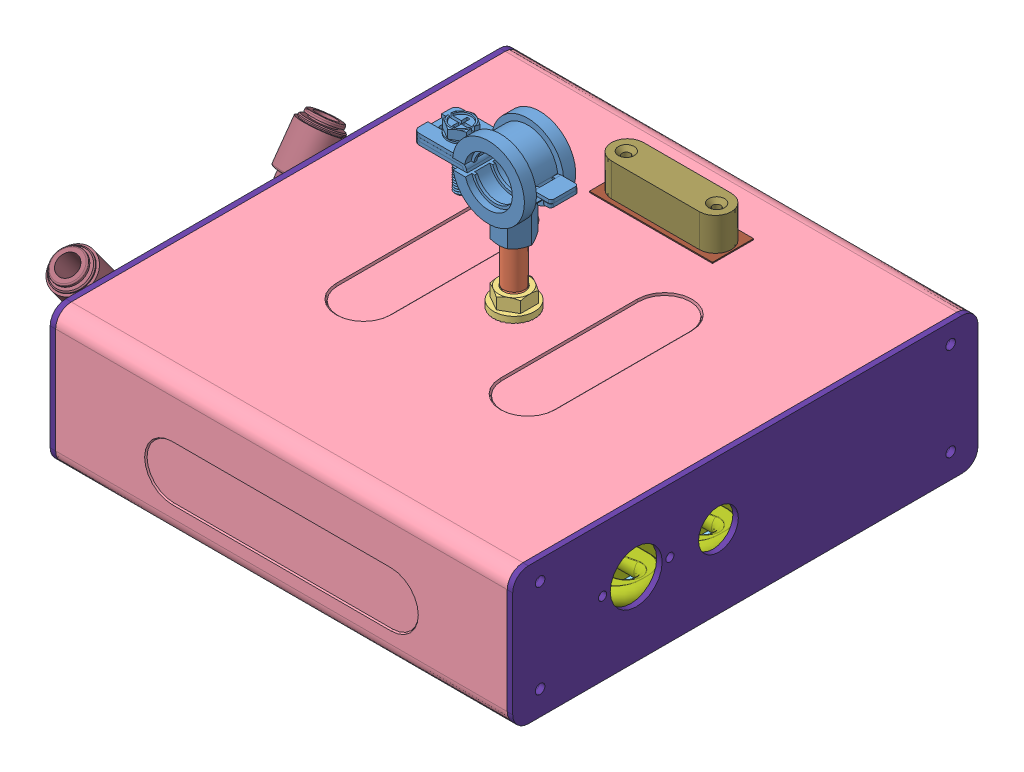
SolidWorks assembly LFR.101, configuration Default. Lengths in mm.
Overall size (264.18 207.36 215.9).
37 component instances, 17 part files, 61 mates.
Components (placement in the parent):
- 2615T130_VIBRATION-DAMPING CLAMPING HANGER-1: 2615T130_VIBRATION-DAMPING CLAMPING HANGER [2615T13] x (-1 0 0) z (0 0 1) size (60.33 44.72 23.81)
- 92386A632_SS THRD-LOCKING ADJUSTING   POSITIONING STUD-1: 92386A632_SS THRD-LOCKING ADJUSTING   POSITIONING STUD [92386A632] at (0 -65.8495 0) x (1 0 0) z (0 -1 0) size (10.08 10.01 51.87)
- 93776A461_TYPE 18-8 SS SERRATED-FLANGE LOCKNUT-1: 93776A461_TYPE 18-8 SS SERRATED-FLANGE LOCKNUT [93776A461] at (0 -47.3075 0) x (1 0 0) z (0 1 0) size (19.05 19.05 9.51)
- LFR.001-1: LFR.001 [BENT] at (0 -56.0388 0) size (209.55 64.1 215.9)
- LightPanel-1: LightPanel [Default] at (5.3651 -116.5988 -8.8508) x (0 0 -1) z (-1 0 0) size (195.78 12.57 210.82)
  - LightPCB-1: LightPCB [Default] at (-97.8524 -1.8098 101.8851) size (195.78 1.57 210.82)
  - KNAC36xxADS_Optic-1: KNAC36xxADS_Optic [Default] at (-8.8508 2.765 90.5129) x (0 0 1) z (0 1 0) size (193.04 178 11)
- aavid_heatsink-1: aavid_heatsink [Default] at (0.2 -114.7889 0) x (-1 0 0) z (0 0 -1) size (237.85 17.03 177.8)
- 92949A133_18-8 SS BUTTON-HEAD SOCKET CAP SCREW-1: 92949A133_18-8 SS BUTTON-HEAD SOCKET CAP SCREW [92949A133] at (100.965 -121.2151 93.4466) x (-0.331806 0 0.943348) z (0 -1 0) size (6.05 6.05 11.55)
- 94241A230_TYPE 316 STAINLESS STEEL SPLIT LOCK WASHER-1: 94241A230_TYPE 316 STAINLESS STEEL SPLIT LOCK WASHER [94241A230] at (100.965 -114.0269 93.4466) x (0.331806 0 -0.943348) z (0 -1 0) size (5.13 5.14 1.64)
- 90730A006_TYPE 18-8 STAINLESS STEEL NARROW HEX NUT-1: 90730A006_TYPE 18-8 STAINLESS STEEL NARROW HEX NUT [90730A006] at (100.965 -111.9978 93.4466) x (0.975805 0 0.218641) z (-0.218641 0 0.975805) size (6.35 2.87 7.33)
- 92949A133_18-8 SS BUTTON-HEAD SOCKET CAP SCREW-4: 92949A133_18-8 SS BUTTON-HEAD SOCKET CAP SCREW [92949A133] at (-100.965 -121.2151 93.4466) x (-0.331806 0 0.943348) z (0 -1 0) size (6.05 6.05 11.55)
- 92949A133_18-8 SS BUTTON-HEAD SOCKET CAP SCREW-5: 92949A133_18-8 SS BUTTON-HEAD SOCKET CAP SCREW [92949A133] at (100.965 -121.2151 -94.0054) x (-0.331806 0 0.943348) z (0 -1 0) size (6.05 6.05 11.55)
- 92949A133_18-8 SS BUTTON-HEAD SOCKET CAP SCREW-8: 92949A133_18-8 SS BUTTON-HEAD SOCKET CAP SCREW [92949A133] at (-100.965 -121.2151 -94.0054) x (-0.331806 0 0.943348) z (0 -1 0) size (6.05 6.05 11.55)
- 90730A006_TYPE 18-8 STAINLESS STEEL NARROW HEX NUT-4: 90730A006_TYPE 18-8 STAINLESS STEEL NARROW HEX NUT [90730A006] at (-100.965 -111.9978 93.4466) x (0.975805 0 0.218641) z (-0.218641 0 0.975805) size (6.35 2.87 7.33)
- 90730A006_TYPE 18-8 STAINLESS STEEL NARROW HEX NUT-5: 90730A006_TYPE 18-8 STAINLESS STEEL NARROW HEX NUT [90730A006] at (100.965 -111.9978 -94.0054) x (0.975805 0 0.218641) z (-0.218641 0 0.975805) size (6.35 2.87 7.33)
- 90730A006_TYPE 18-8 STAINLESS STEEL NARROW HEX NUT-8: 90730A006_TYPE 18-8 STAINLESS STEEL NARROW HEX NUT [90730A006] at (-100.965 -111.9978 -94.0054) x (0.975805 0 0.218641) z (-0.218641 0 0.975805) size (6.35 2.87 7.33)
- 94241A230_TYPE 316 STAINLESS STEEL SPLIT LOCK WASHER-4: 94241A230_TYPE 316 STAINLESS STEEL SPLIT LOCK WASHER [94241A230] at (-100.965 -114.0269 93.4466) x (0.331806 0 -0.943348) z (0 -1 0) size (5.13 5.14 1.64)
- 94241A230_TYPE 316 STAINLESS STEEL SPLIT LOCK WASHER-5: 94241A230_TYPE 316 STAINLESS STEEL SPLIT LOCK WASHER [94241A230] at (100.965 -114.0269 -94.0054) x (0.331806 0 -0.943348) z (0 -1 0) size (5.13 5.14 1.64)
- 94241A230_TYPE 316 STAINLESS STEEL SPLIT LOCK WASHER-8: 94241A230_TYPE 316 STAINLESS STEEL SPLIT LOCK WASHER [94241A230] at (-100.965 -114.0269 -94.0054) x (0.331806 0 -0.943348) z (0 -1 0) size (5.13 5.14 1.64)
- 76665A68_VHB_TAPE-1: 76665A68_VHB_TAPE [Default] at (0 -56.0388 -73.025) x (0 0 1) z (-1 0 0) size (19.05 0.51 57.15)
- 3338A22_HORIZONTAL_SURFACE_MOUNT_LEVEL-1: 3338A22_HORIZONTAL_SURFACE_MOUNT_LEVEL [Default] at (0.0625 -55.5307 -72.9641) size (55.63 15.24 14.83)
- 9406T170_PUSH-TO-CONNECT TUBE FITTING FOR SS TUBING-1: 9406T170_PUSH-TO-CONNECT TUBE FITTING FOR SS TUBING [9406T17] at (-147.214 -103.439 -45.2) x (0 -0.582087 -0.813127) z (1 0 0) size (19.3 35.05 39.88)
- 9406T170_PUSH-TO-CONNECT TUBE FITTING FOR SS TUBING-2: 9406T170_PUSH-TO-CONNECT TUBE FITTING FOR SS TUBING [9406T17] at (-147.214 -103.439 45) x (0 0.587828 -0.808986) z (1 0 0) size (19.3 35.05 39.88)
- 94639A303_NYLON UNTHREADED SPACERS-1: 94639A303_NYLON UNTHREADED SPACERS [94639A303] at (-40.44 -94.4389 -55.499) x (0.961212 0 0.275811) z (0 1 0) size (6.35 6.35 12.7)
- 94639A303_NYLON UNTHREADED SPACERS-2: 94639A303_NYLON UNTHREADED SPACERS [94639A303] at (40.84 -94.4389 -55.499) x (0.961212 0 0.275811) z (0 1 0) size (6.35 6.35 12.7)
- 94639A303_NYLON UNTHREADED SPACERS-3: 94639A303_NYLON UNTHREADED SPACERS [94639A303] at (40.84 -94.4389 55.499) x (0.961212 0 0.275811) z (0 1 0) size (6.35 6.35 12.7)
- 94639A303_NYLON UNTHREADED SPACERS-4: 94639A303_NYLON UNTHREADED SPACERS [94639A303] at (-40.44 -94.4389 55.499) x (0.961212 0 0.275811) z (0 1 0) size (6.35 6.35 12.7)
- 92949A151_18-8 SS BUTTON-HEAD SOCKET CAP SCREW-1: 92949A151_18-8 SS BUTTON-HEAD SOCKET CAP SCREW [92949A151] at (-40.44 -84.4567 -55.499) x (0.994916 0 -0.100706) z (0 1 0) size (6.65 6.65 21.35)
- 92949A151_18-8 SS BUTTON-HEAD SOCKET CAP SCREW-2: 92949A151_18-8 SS BUTTON-HEAD SOCKET CAP SCREW [92949A151] at (-40.44 -84.4567 55.499) x (0.991359 0 -0.131179) z (0 1 0) size (6.65 6.65 21.35)
- 92949A151_18-8 SS BUTTON-HEAD SOCKET CAP SCREW-3: 92949A151_18-8 SS BUTTON-HEAD SOCKET CAP SCREW [92949A151] at (40.84 -84.4567 55.499) x (0.991359 0 -0.131179) z (0 1 0) size (6.65 6.65 21.35)
- 92949A151_18-8 SS BUTTON-HEAD SOCKET CAP SCREW-4: 92949A151_18-8 SS BUTTON-HEAD SOCKET CAP SCREW [92949A151] at (40.84 -84.4567 -55.499) x (0.991359 0 -0.131179) z (0 1 0) size (6.65 6.65 21.35)
- light_controller v16-1: light_controller v16 [Default] at (-45.52 -88.0889 -60.579) x (0 0 1) z (0 1 0) size (121.16 91.44 17.03)
- LFR.008-1: LFR.008 [Front-1] at (-102.235 -158.9087 0) x (0 0 1) z (-1 0 0) size (215.9 131.44 2.54)
- LFR.008-2: LFR.008 [Front-2] at (-104.775 -87.7887 0) x (0 0 1) z (-1 0 0) size (215.9 131.44 2.54)
- LFR.008-3: LFR.008 [Back1] at (104.775 -158.9087 0) x (0 0 1) z (-1 0 0) size (215.9 131.44 2.54)
- LFR.008-4: LFR.008 [Back2] at (107.315 -87.7887 0) x (0 0 1) z (-1 0 0) size (215.9 131.44 2.54)
Mates (geometry in assembly coordinates):
- Coincident1: coincident: plane of 2615T130_VIBRATION-DAMPING CLAMPING HANGER-1 through (0 0 0) normal (0 0 1); plane of assembly through (0 0 0) normal (0 0 1)
- Coincident2: coincident: plane of 2615T130_VIBRATION-DAMPING CLAMPING HANGER-1 through (0 0 0) normal (0 -1 0); plane of assembly through (0 0 0) normal (0 1 0)
- Coincident3: coincident: plane of 2615T130_VIBRATION-DAMPING CLAMPING HANGER-1 through (0 0 0) normal (-1 0 0); plane of assembly through (0 0 0) normal (1 0 0)
- Concentric1: concentric: cylinder of 2615T130_VIBRATION-DAMPING CLAMPING HANGER-1 through (0 16.7015 0) axis (0 -1 0) radius 5.3975; cylinder of 92386A632_SS THRD-LOCKING ADJUSTING   POSITIONING STUD-1 through (0 -15.0495 0) axis (0 1 0) radius 4.7625
- Coincident4: coincident: plane of 2615T130_VIBRATION-DAMPING CLAMPING HANGER-1 through (-8.1389 -27.7495 0) normal (0 -1 0); plane of 92386A632_SS THRD-LOCKING ADJUSTING   POSITIONING STUD-1 through (0 -27.7495 0) normal (0 1 0)
- Concentric2: concentric: cylinder of LFR.001-1 through (0 -59.2138 0) axis (0 -1 0) radius 7.112; cylinder of 92386A632_SS THRD-LOCKING ADJUSTING   POSITIONING STUD-1 through (0 -15.0495 0) axis (0 1 0) radius 4.7625
- Concentric3: concentric: cylinder of 93776A461_TYPE 18-8 SS SERRATED-FLANGE LOCKNUT-1 through (0 -53.0669 0) axis (0 -1 0) radius 9.525; cylinder of 92386A632_SS THRD-LOCKING ADJUSTING   POSITIONING STUD-1 through (0 -15.0495 0) axis (0 1 0) radius 4.7625
- Coincident5: coincident: plane of LFR.001-1 through (-104.775 -56.0388 107.95) normal (0 1 0); point of 93776A461_TYPE 18-8 SS SERRATED-FLANGE LOCKNUT-1
- Parallel1: parallel: plane of 2615T130_VIBRATION-DAMPING CLAMPING HANGER-1 through (-36.83 -3.1877 33.5953) normal (-1 0 0); plane of LFR.001-1 through (-104.775 -59.2138 107.95) normal (-1 0 0)
- Distance1: distance = 0.508 mm: plane of 93776A461_TYPE 18-8 SS SERRATED-FLANGE LOCKNUT-1 through (-7.1437 -47.3075 -12.3733) normal (0 1 0); plane of 92386A632_SS THRD-LOCKING ADJUSTING   POSITIONING STUD-1 through (0 -46.7995 0) normal (0 -1 0)
- Coincident6: coincident: plane of LightPanel-1/LightPCB-1 through (-96.52 -114.7889 89.0016) normal (0 1 0); plane of aavid_heatsink-1 through (0.2 -114.7889 0) normal (0 -1 0)
- Distance2: distance = 29.21 mm: plane of aavid_heatsink-1 through (76.2 -100.7889 88.9) normal (1 0 0); plane of LightPanel-1/LightPCB-1 through (105.41 -116.3637 -97.8916) normal (1 0 0)
- Coincident8: coincident: plane of LFR.001-1 through (0 -116.3637 0) normal (0 1 0); plane of LightPanel-1/LightPCB-1 through (-96.52 -116.3637 89.0016) normal (0 -1 0)
- Width3: width: plane of aavid_heatsink-1 through (76.2 -100.7889 -88.9) normal (0 0 -1); plane of aavid_heatsink-1 through (76.2 -100.7889 88.9) normal (0 0 1); plane of LightPanel-1/LightPCB-1 through (105.41 -116.3637 97.8916) normal (0 0 1); plane of LightPanel-1/LightPCB-1 through (-105.41 -116.3637 -97.8916) normal (0 0 -1)
- Parallel2: parallel: plane of LFR.001-1 through (104.775 -56.0388 107.95) normal (1 0 0); plane of aavid_heatsink-1 through (76.2 -100.7889 88.9) normal (1 0 0)
- Width4: width: plane of LFR.001-1 through (0 -56.0388 107.95) normal (0 0 1); plane of LFR.001-1 through (0 -56.0388 -107.95) normal (0 0 -1); plane of aavid_heatsink-1 through (76.2 -100.7889 -88.9) normal (0 0 -1); plane of aavid_heatsink-1 through (76.2 -100.7889 88.9) normal (0 0 1)
- Width5: width: plane of LightPanel-1/LightPCB-1 through (105.41 -116.3637 -97.8916) normal (1 0 0); plane of LightPanel-1/LightPCB-1 through (-105.41 -116.3637 97.8916) normal (-1 0 0); plane of LFR.001-1 through (104.775 -59.2138 107.95) normal (1 0 0); plane of LFR.001-1 through (-104.775 -119.5387 107.95) normal (-1 0 0)
- Concentric4: concentric: cylinder of LightPanel-1/LightPCB-1 through (100.965 -116.3637 93.4466) axis (0 1 0) radius 1.778; cylinder of 92949A133_18-8 SS BUTTON-HEAD SOCKET CAP SCREW-1 through (100.965 -121.2151 93.4466) axis (0 -1 0) radius 3.0226
- Coincident11: coincident: plane of LightPanel-1/LightPCB-1 through (-96.52 -114.7889 89.0016) normal (0 1 0); point of 94241A230_TYPE 316 STAINLESS STEEL SPLIT LOCK WASHER-1
- Parallel3: parallel: plane of LightPanel-1/LightPCB-1 through (-96.52 -114.7889 89.0016) normal (0 1 0); plane of 94241A230_TYPE 316 STAINLESS STEEL SPLIT LOCK WASHER-1 through (100.965 -114.0269 93.4466) normal (0 -1 0)
- Coincident13: coincident: plane of 92949A133_18-8 SS BUTTON-HEAD SOCKET CAP SCREW-1 through (100.965 -121.2151 93.4466) normal (-0.331806 0 0.943348); plane of 94241A230_TYPE 316 STAINLESS STEEL SPLIT LOCK WASHER-1 through (100.965 -114.0269 93.4466) normal (0.331806 0 -0.943348)
- Coincident14: coincident: plane of 92949A133_18-8 SS BUTTON-HEAD SOCKET CAP SCREW-1 through (100.965 -121.2151 93.4466) normal (-0.943348 0 -0.331806); plane of 94241A230_TYPE 316 STAINLESS STEEL SPLIT LOCK WASHER-1 through (100.965 -114.0269 93.4466) normal (0.943348 0 0.331806)
- Coincident15: coincident: plane of LFR.001-1 through (0 -119.5387 0) normal (0 -1 0); plane of 92949A133_18-8 SS BUTTON-HEAD SOCKET CAP SCREW-1 through (103.8164 -119.5387 94.4495) normal (0 1 0)
- Concentric5: concentric: cylinder of 92949A133_18-8 SS BUTTON-HEAD SOCKET CAP SCREW-1 through (100.965 -121.2151 93.4466) axis (0 -1 0) radius 3.0226; circle of 90730A006_TYPE 18-8 STAINLESS STEEL NARROW HEX NUT-1
- Coincident16: coincident: point of 94241A230_TYPE 316 STAINLESS STEEL SPLIT LOCK WASHER-1; plane of 90730A006_TYPE 18-8 STAINLESS STEEL NARROW HEX NUT-1 through (98.2676 -113.1884 90.9637) normal (0 -1 0)
- Coincident17: coincident: plane of LFR.001-1 through (-104.775 -56.0388 107.95) normal (0 1 0); plane of 76665A68_VHB_TAPE-1 through (0 -56.0388 -73.025) normal (0 -1 0)
- Distance3: distance = 25.4 mm: plane of 76665A68_VHB_TAPE-1 through (28.575 -55.5307 -82.55) normal (0 0 -1); plane of LFR.001-1 through (0 -56.0388 -107.95) normal (0 0 -1)
- Width6: width: plane of 76665A68_VHB_TAPE-1 through (-28.575 -55.5307 -82.55) normal (-1 0 0); plane of 76665A68_VHB_TAPE-1 through (28.575 -55.5307 -82.55) normal (1 0 0); plane of LFR.001-1 through (104.775 -56.0388 107.95) normal (1 0 0); plane of LFR.001-1 through (-104.775 -59.2138 107.95) normal (-1 0 0)
- Coincident19: coincident: plane of 76665A68_VHB_TAPE-1 through (0 -55.5307 -73.025) normal (0 1 0); plane of 3338A22_HORIZONTAL_SURFACE_MOUNT_LEVEL-1 through (-20.3337 -55.5307 -72.9641) normal (0 -1 0)
- Concentric6: concentric: cylinder of aavid_heatsink-1 through (87.28 -103.439 -45.2) axis (-1 0 0) radius 4.75; cylinder of 9406T170_PUSH-TO-CONNECT TUBE FITTING FOR SS TUBING-1 through (-116.988 -103.439 -45.2) axis (1 0 0) radius 4.7625
- Coincident20: coincident: plane of aavid_heatsink-1 through (-136.8 -103.439 -45.2) normal (-1 0 0); plane of 9406T170_PUSH-TO-CONNECT TUBE FITTING FOR SS TUBING-1 through (-136.8 -99.5664 -47.9722) normal (1 0 0)
- Coincident21: coincident: plane of 9406T170_PUSH-TO-CONNECT TUBE FITTING FOR SS TUBING-1 through (-139.2765 -97.1138 -49.7279) normal (-1 0 0); plane of 9406T170_PUSH-TO-CONNECT TUBE FITTING FOR SS TUBING-2 through (-139.2765 -97.146 49.5726) normal (-1 0 0)
- Concentric7: concentric: cylinder of aavid_heatsink-1 through (87.28 -103.439 45) axis (-1 0 0) radius 4.75; cylinder of 9406T170_PUSH-TO-CONNECT TUBE FITTING FOR SS TUBING-2 through (-116.988 -103.439 45) axis (1 0 0) radius 9.652
- Concentric8: concentric: cylinder of aavid_heatsink-1 through (-40.44 -113.489 -55.499) axis (0 1 0) radius 1.3526; cylinder of ? through (-40.44 -88.0889 -55.499) axis (0 -1 0) radius 3.175
- Coincident22: coincident: plane of aavid_heatsink-1 through (0.2 -100.7889 0) normal (0 1 0); plane of ? through (-40.44 -100.7889 -55.499) normal (0 -1 0)
- Coincident23: coincident: plane of ? through (-40.44 -88.0889 -55.499) normal (0 1 0); plane of 94639A303_NYLON UNTHREADED SPACERS-4 through (-40.44 -88.0889 55.499) normal (0 1 0)
- Coincident24: coincident: plane of ? through (40.84 -88.0889 -55.499) normal (0 1 0); plane of 94639A303_NYLON UNTHREADED SPACERS-3 through (40.84 -88.0889 55.499) normal (0 1 0)
- Coincident25: coincident: plane of 94639A303_NYLON UNTHREADED SPACERS-3 through (40.84 -88.0889 55.499) normal (0 1 0); plane of 94639A303_NYLON UNTHREADED SPACERS-4 through (-40.44 -88.0889 55.499) normal (0 1 0)
- Concentric9: concentric: cylinder of aavid_heatsink-1 through (40.84 -113.489 -55.499) axis (0 1 0) radius 1.3526; cylinder of ? through (40.84 -88.0889 -55.499) axis (0 -1 0) radius 3.175
- Concentric10: concentric: cylinder of aavid_heatsink-1 through (-40.44 -113.489 55.499) axis (0 1 0) radius 1.3526; cylinder of 94639A303_NYLON UNTHREADED SPACERS-4 through (-40.44 -88.0889 55.499) axis (0 -1 0) radius 3.175
- Concentric11: concentric: cylinder of aavid_heatsink-1 through (40.84 -113.489 55.499) axis (0 1 0) radius 1.3526; cylinder of 94639A303_NYLON UNTHREADED SPACERS-3 through (40.84 -88.0889 55.499) axis (0 -1 0) radius 3.175
- Concentric12: concentric: cylinder of ? through (-40.44 -88.0889 -55.499) axis (0 -1 0) radius 3.175; cylinder of ? through (-40.44 -84.4567 -55.499) axis (0 1 0) radius 3.3274
- Coincident26: coincident: plane of ? through (-40.1049 -86.3109 -52.1885) normal (0 -1 0); plane of 92949A151_18-8 SS BUTTON-HEAD SOCKET CAP SCREW-3 through (41.2765 -86.3109 58.7976) normal (0 -1 0)
- Coincident27: coincident: plane of 92949A151_18-8 SS BUTTON-HEAD SOCKET CAP SCREW-3 through (41.2765 -86.3109 58.7976) normal (0 -1 0); plane of ? through (41.2765 -86.3109 -52.2004) normal (0 -1 0)
- Coincident28: coincident: plane of 92949A151_18-8 SS BUTTON-HEAD SOCKET CAP SCREW-2 through (-40.0035 -86.3109 58.7976) normal (0 -1 0); plane of ? through (41.2765 -86.3109 -52.2004) normal (0 -1 0)
- Concentric13: concentric: cylinder of 94639A303_NYLON UNTHREADED SPACERS-3 through (40.84 -88.0889 55.499) axis (0 -1 0) radius 3.175; cylinder of 92949A151_18-8 SS BUTTON-HEAD SOCKET CAP SCREW-3 through (40.84 -84.4567 55.499) axis (0 1 0) radius 3.3274
- Concentric14: concentric: cylinder of ? through (40.84 -88.0889 -55.499) axis (0 -1 0) radius 3.175; cylinder of ? through (40.84 -84.4567 -55.499) axis (0 1 0) radius 3.3274
- Concentric15: concentric: cylinder of 94639A303_NYLON UNTHREADED SPACERS-4 through (-40.44 -88.0889 55.499) axis (0 -1 0) radius 3.175; cylinder of 92949A151_18-8 SS BUTTON-HEAD SOCKET CAP SCREW-2 through (-40.44 -84.4567 55.499) axis (0 1 0) radius 3.3274
- Distance4: distance = 1.778 mm: plane of 92949A151_18-8 SS BUTTON-HEAD SOCKET CAP SCREW-1 through (-40.1049 -86.3109 -52.1885) normal (0 -1 0); plane of 94639A303_NYLON UNTHREADED SPACERS-1 through (-40.44 -88.0889 -55.499) normal (0 1 0)
- Concentric20: concentric: cylinder of LFR.008-1 through (-104.775 -103.439 -45.2) axis (1 0 0) radius 5.08; cylinder of LFR.008-2 through (-107.315 -103.439 -45.2) axis (1 0 0) radius 5.08
- Coincident31: coincident: plane of LFR.008-1 through (-104.775 -63.2777 100.711) normal (-1 0 0); plane of LFR.008-2 through (-104.775 -63.2777 -100.711) normal (1 0 0)
- Coincident32: coincident: plane of LFR.001-1 through (-104.775 -59.2138 -107.95) normal (-1 0 0); plane of LFR.008-2 through (-104.775 -63.2777 -100.711) normal (1 0 0)
- Concentric21: concentric: cylinder of aavid_heatsink-1 through (87.28 -103.439 45) axis (-1 0 0) radius 4.75; cylinder of LFR.008-2 through (-107.315 -103.439 45) axis (1 0 0) radius 5.08
- Concentric22: concentric: cylinder of aavid_heatsink-1 through (87.28 -103.439 45) axis (-1 0 0) radius 4.75; cylinder of LFR.008-1 through (-104.775 -103.439 45) axis (1 0 0) radius 5.08
- Concentric23: concentric: cylinder of aavid_heatsink-1 through (87.28 -103.439 -45.2) axis (-1 0 0) radius 4.75; cylinder of LFR.008-2 through (-107.315 -103.439 -45.2) axis (1 0 0) radius 5.08
- Coincident34: coincident: plane of LFR.008-2 through (-107.315 -63.2777 -107.95) normal (0 0 -1); plane of LFR.008-4 through (104.775 -63.2777 -107.95) normal (0 0 -1)
- Coincident35: coincident: plane of LFR.008-2 through (-107.315 -119.5387 52.4295) normal (0 -1 0); plane of LFR.008-4 through (104.775 -119.5387 52.4295) normal (0 -1 0)
- Coincident37: coincident: plane of LFR.008-3 through (104.775 -63.2777 100.711) normal (1 0 0); plane of LFR.008-4 through (104.775 -63.2777 -100.711) normal (-1 0 0)
- Width8: width: plane of LFR.008-4 through (104.775 -112.2998 107.95) normal (0 0 1); plane of LFR.008-4 through (104.775 -63.2777 -107.95) normal (0 0 -1); plane of LFR.008-3 through (102.235 -63.2777 -104.775) normal (0 0 -1); plane of LFR.008-3 through (102.235 -108.5637 104.775) normal (0 0 1)
- Coincident40: coincident: plane of LFR.001-1 through (-104.775 -59.2138 107.95) normal (0 -1 0); plane of LFR.008-3 through (102.235 -59.2138 100.711) normal (0 1 0)
- Coincident41: coincident: plane of LFR.001-1 through (104.775 -119.5387 104.775) normal (1 0 0); plane of LFR.008-4 through (104.775 -63.2777 -100.711) normal (-1 0 0)
